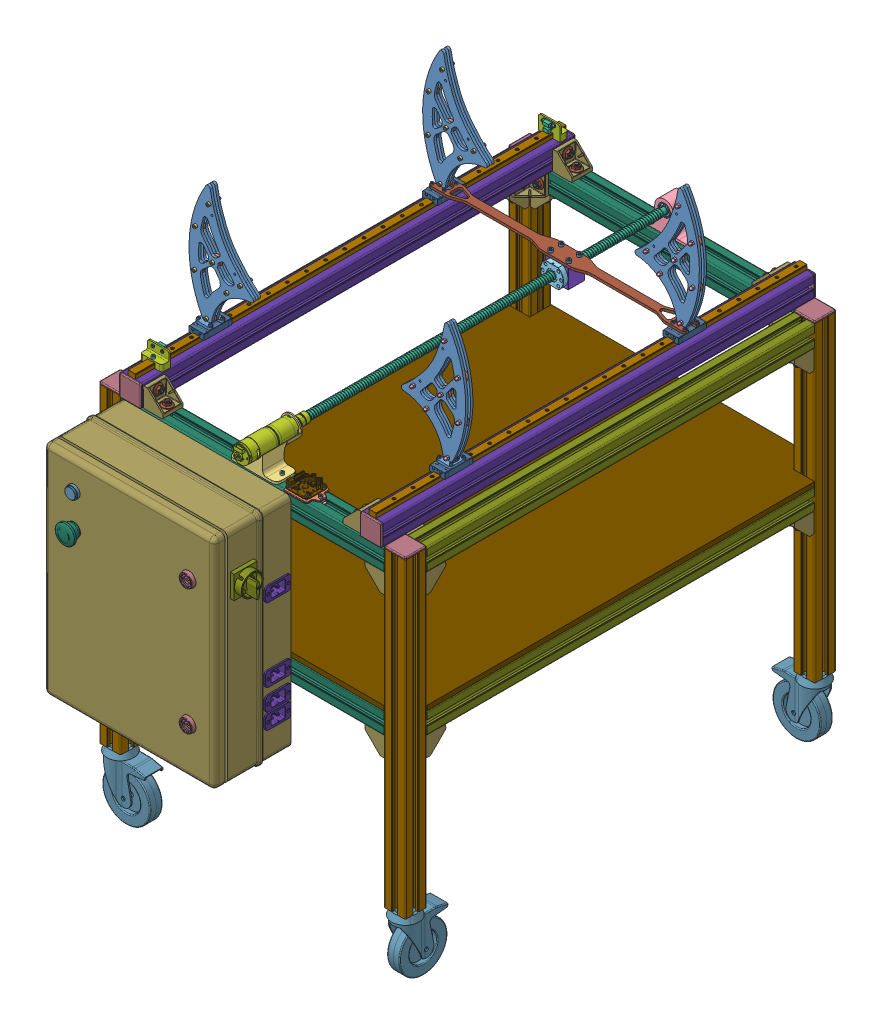
SolidWorks assembly Montaje_Eje_Z, configuration Predeterminado. Lengths in mm.
Overall size (651 1094.15 1088.52).
428 component instances, 43 part files, 191 mates.
Components (placement in the parent):
- socket head cap screw_iso2-2: socket head cap screw_iso2 [ISO 4762 M3 x 8 - 8N] at (-240.4498 15.8322 -56.4995) x (0 -1 0) z (0 0 1) size (11 5.5 5.5)
- socket head cap screw_iso2-3: socket head cap screw_iso2 [ISO 4762 M3 x 8 - 8N] at (-215.4498 15.8322 -31.4995) x (0 -1 0) z (0 0 1) size (11 5.5 5.5)
- socket head cap screw_iso2-4: socket head cap screw_iso2 [ISO 4762 M3 x 8 - 8N] at (-240.4498 15.8322 -31.4995) x (0 -1 0) z (0 0 1) size (11 5.5 5.5)
- socket head cap screw_iso2-5: socket head cap screw_iso2 [ISO 4762 M3 x 8 - 8N] at (-215.4498 15.8322 -56.4995) x (0 -1 0) z (0.194661 0 0.98087) size (11 5.5 5.5)
- socket head cap screw_iso2-6: socket head cap screw_iso2 [ISO 4762 M3 x 8 - 8N] at (287.5502 15.8322 -56.4995) x (0 -1 0) z (0.194661 0 0.98087) size (11 5.5 5.5)
- socket head cap screw_iso2-7: socket head cap screw_iso2 [ISO 4762 M3 x 8 - 8N] at (262.5502 15.8322 -31.4995) x (0 -1 0) z (0 0 1) size (11 5.5 5.5)
- socket head cap screw_iso2-8: socket head cap screw_iso2 [ISO 4762 M3 x 8 - 8N] at (287.5502 15.8322 -31.4995) x (0 -1 0) z (-0.140271 0 0.990113) size (11 5.5 5.5)
- socket head cap screw_iso2-9: socket head cap screw_iso2 [ISO 4762 M3 x 8 - 8N] at (262.5502 15.8322 -56.4995) x (0 -1 0) z (-0.070011 0 0.997546) size (11 5.5 5.5)
- socket head cap screw_iso2-10: socket head cap screw_iso2 [ISO 4762 M5 x 16 - 16N] at (43.5502 17.8322 -54.9995) x (0 -1 0) z (0 0 1) size (21 8.5 8.5)
- socket head cap screw_iso2-11: socket head cap screw_iso2 [ISO 4762 M5 x 16 - 16N] at (43.5502 17.8322 -32.9995) x (0 -1 0) z (0.965322 0 -0.261062) size (21 8.5 8.5)
- socket head cap screw_iso2-12: socket head cap screw_iso2 [ISO 4762 M5 x 16 - 16N] at (5.5502 17.8322 -32.9995) x (0 -1 0) z (0 0 1) size (21 8.5 8.5)
- socket head cap screw_iso2-13: socket head cap screw_iso2 [ISO 4762 M5 x 16 - 16N] at (5.5502 17.8322 -54.9995) x (0 -1 0) z (0 0 1) size (21 8.5 8.5)
- socket head cap screw_iso2-23: socket head cap screw_iso2 [ISO 4762 M3 x 8 - 8N] at (287.5502 15.8322 456.5005) x (0 -1 0) z (0 0 1) size (11 5.5 5.5)
- socket head cap screw_iso2-24: socket head cap screw_iso2 [ISO 4762 M3 x 8 - 8N] at (287.5502 15.8322 431.5005) x (0 -1 0) z (0 0 1) size (11 5.5 5.5)
- socket head cap screw_iso2-25: socket head cap screw_iso2 [ISO 4762 M3 x 8 - 8N] at (262.5502 15.8322 456.5005) x (0 -1 0) z (0 0 1) size (11 5.5 5.5)
- socket head cap screw_iso2-26: socket head cap screw_iso2 [ISO 4762 M3 x 8 - 8N] at (262.5502 15.8322 431.5005) x (0 -1 0) z (0 0 1) size (11 5.5 5.5)
- socket head cap screw_iso2-27: socket head cap screw_iso2 [ISO 4762 M3 x 8 - 8N] at (-240.4501 15.8323 456.5005) x (0 -1 0) z (0 0 1) size (11 5.5 5.5)
- socket head cap screw_iso2-28: socket head cap screw_iso2 [ISO 4762 M3 x 8 - 8N] at (-215.4501 15.8323 456.5005) x (0 -1 0) z (0 0 1) size (11 5.5 5.5)
- socket head cap screw_iso2-29: socket head cap screw_iso2 [ISO 4762 M3 x 8 - 8N] at (-240.4501 15.8323 431.5005) x (0 -1 0) z (0 0 1) size (11 5.5 5.5)
- socket head cap screw_iso2-30: socket head cap screw_iso2 [ISO 4762 M3 x 8 - 8N] at (-215.4501 15.8323 431.5005) x (0 -1 0) z (0 0 1) size (11 5.5 5.5)
- socket head cap screw_iso2-31: socket head cap screw_iso2 [ISO 4762 M4 x 8 - 8N] at (144.6751 -48.9678 586.0585) x (0 -1 0) z (0 0 1) size (12 7 7)
- socket head cap screw_iso2-33: socket head cap screw_iso2 [ISO 4762 M4 x 8 - 8N] at (84.6751 -48.9678 586.0585) x (0 -1 0) z (0 0 1) size (12 7 7)
- hexa csunk flathd screw_iso2-1: hexa csunk flathd screw_iso2 [ISO 14581 M3x12x12-N] at (133.4451 -55.9678 604.7785) x (-0.795034 0 0.606565) z (0 -1 0) size (5.5 5.5 12)
- hexa csunk flathd screw_iso2-2: hexa csunk flathd screw_iso2 [ISO 14581 M3x12x12-N] at (96.0351 -55.9678 604.7785) x (-0.795034 0 0.606565) z (0 -1 0) size (5.5 5.5 12)
- hexa csunk flathd screw_iso2-4: hexa csunk flathd screw_iso2 [ISO 14581 M3x12x12-N] at (133.4451 -55.9678 567.3685) x (-0.795034 0 0.606565) z (0 -1 0) size (5.5 5.5 12)
- hexa csunk flathd screw_iso2-5: hexa csunk flathd screw_iso2 [ISO 14581 M3x12x12-N] at (96.0351 -55.9678 567.3685) x (-0.795034 0 0.606565) z (0 -1 0) size (5.5 5.5 12)
- hex thin nut chamfered gradeab_iso-1: hex thin nut chamfered gradeab_iso [ISO - 4035 - M3 - N] at (96.0351 -46.1293 604.7785) x (0.635839 0 0.771821) z (0 1 0) size (5.5 6.35 1.8)
- hex thin nut chamfered gradeab_iso-2: hex thin nut chamfered gradeab_iso [ISO - 4035 - M3 - N] at (133.4739 -46.1293 604.6517) x (1 0 0) z (0 1 0) size (5.5 6.35 1.8)
- hex thin nut chamfered gradeab_iso-3: hex thin nut chamfered gradeab_iso [ISO - 4035 - M3 - N] at (133.4739 -46.1293 567.2883) x (1 0 0) z (0 1 0) size (5.5 6.35 1.8)
- hex thin nut chamfered gradeab_iso-4: hex thin nut chamfered gradeab_iso [ISO - 4035 - M3 - N] at (96.0597 -46.1293 567.2629) x (1 0 0) z (0 1 0) size (5.5 6.35 1.8)
- bosch_3842530281_56mh0c106byol9t07uu6uwj7k-1: bosch_3842530281_56mh0c106byol9t07uu6uwj7k [Default] at (84.6751 -58.9678 586.0585) x (1 0 0) z (0 0 1) size (19.6 8.7 10)
- bosch_3842530281_56mh0c106byol9t07uu6uwj7k-2: bosch_3842530281_56mh0c106byol9t07uu6uwj7k [Default] at (144.6751 -58.9678 586.0585) x (1 0 0) z (0 0 1) size (19.6 8.7 10)
- bosch_3842530281_56mh0c106byol9t07uu6uwj7k-3: bosch_3842530281_56mh0c106byol9t07uu6uwj7k [Default] at (64.0502 -58.9678 586.0585) x (1 0 0) z (0 0 1) size (19.6 8.7 10)
- bosch_3842530281_56mh0c106byol9t07uu6uwj7k-4: bosch_3842530281_56mh0c106byol9t07uu6uwj7k [Default] at (-14.9498 -58.9678 586.0585) x (1 0 0) z (0 0 1) size (19.6 8.7 10)
- socket head cap screw_iso-1: socket head cap screw_iso [ISO 4762 M4 x 8 - 8N] at (64.0502 -46.9678 586.0585) x (0 -1 0) z (0 0 1) size (12 7 7)
- socket head cap screw_iso-2: socket head cap screw_iso [ISO 4762 M4 x 8 - 8N] at (-14.9498 -46.9678 586.0585) x (0 -1 0) z (0 0 1) size (12 7 7)
- bosch_3842530281_56mh0c106byol9t07uu6uwj7k-5: bosch_3842530281_56mh0c106byol9t07uu6uwj7k [Default] at (64.5502 -58.9678 -268.9416) x (1 0 0) z (0 0 1) size (19.6 8.7 10)
- bosch_3842530281_56mh0c106byol9t07uu6uwj7k-6: bosch_3842530281_56mh0c106byol9t07uu6uwj7k [Default] at (-15.4498 -58.9678 -268.9416) x (1 0 0) z (0 0 1) size (19.6 8.7 10)
- socket head cap screw_iso-3: socket head cap screw_iso [ISO 4762 M4 x 8 - 8N] at (64.5502 -46.9678 -268.9416) x (0 -1 0) z (0 0 1) size (12 7 7)
- socket head cap screw_iso-4: socket head cap screw_iso [ISO 4762 M4 x 8 - 8N] at (-15.4498 -46.9678 -268.9416) x (0 -1 0) z (0 0 1) size (12 7 7)
- bosch_3842530281_56mh0c106byol9t07uu6uwj7k-7: bosch_3842530281_56mh0c106byol9t07uu6uwj7k [Default] at (-227.9501 -13.9677 -276.5915) x (0 0 1) z (-1 0 0) size (19.6 8.7 10)
- bosch_3842530281_56mh0c106byol9t07uu6uwj7k-8: bosch_3842530281_56mh0c106byol9t07uu6uwj7k [Default] at (-227.9501 -13.9677 563.4085) x (0 0 1) z (-1 0 0) size (19.6 8.7 10)
- bosch_3842530281_56mh0c106byol9t07uu6uwj7k-9: bosch_3842530281_56mh0c106byol9t07uu6uwj7k [Default] at (275.0502 -13.9677 563.7084) x (0 0 -1) z (1 0 0) size (19.6 8.7 10)
- bosch_3842530281_56mh0c106byol9t07uu6uwj7k-10: bosch_3842530281_56mh0c106byol9t07uu6uwj7k [Default] at (275.0502 -13.9677 -276.2916) x (0.798528 0 0.601957) z (-0.601957 0 0.798528) size (19.6 8.7 10)
- socket head cap screw_iso-5: socket head cap screw_iso [ISO 4762 M4 x 16 - 16N] at (-227.9501 6.0323 -276.5915) x (0 -1 0) z (0 0 1) size (20 7 7)
- socket head cap screw_iso-8: socket head cap screw_iso [ISO 4762 M3 x 8 - 8N] at (-237.9501 14.0323 -258.9915) x (0 0 -1) z (1 0 0) size (11 5.5 5.5)
- socket head cap screw_iso-9: socket head cap screw_iso [ISO 4762 M3 x 8 - 8N] at (-217.9501 14.0323 -258.9915) x (0 0 -1) z (1 0 0) size (11 5.5 5.5)
- socket head cap screw_iso-10: socket head cap screw_iso [ISO 4762 M3 x 8 - 8N] at (-217.9501 14.0323 545.8085) x (0 0 1) z (0.923728 0.383049 0) size (11 5.5 5.5)
- socket head cap screw_iso-11: socket head cap screw_iso [ISO 4762 M3 x 8 - 8N] at (-237.9501 14.0323 545.8085) x (0 0 1) z (0.923728 0.383049 0) size (11 5.5 5.5)
- socket head cap screw_iso-12: socket head cap screw_iso [ISO 4762 M4 x 16 - 16N] at (-227.9501 6.0323 563.4085) x (0 -1 0) z (0 0 1) size (20 7 7)
- hex thin nut gradeb_iso-1: hex thin nut gradeb_iso [ISO - 4036 - M3 - N] at (-237.9501 14.0323 555.2085) x (1 0 0) z (0 0 1) size (5.5 6.35 1.8)
- hex thin nut gradeb_iso-2: hex thin nut gradeb_iso [ISO - 4036 - M3 - N] at (-217.9501 14.0323 555.2085) x (1 0 0) z (0 0 1) size (5.5 6.35 1.8)
- hex thin nut gradeb_iso-3: hex thin nut gradeb_iso [ISO - 4036 - M3 - N] at (-237.9501 14.0323 -268.3915) x (-1 -0.000019 0) z (0 0 -1) size (5.5 6.35 1.8)
- hex thin nut gradeb_iso-4: hex thin nut gradeb_iso [ISO - 4036 - M3 - N] at (-217.9501 14.0323 -268.3915) x (-1 -0.000027 0) z (0 0 -1) size (5.5 6.35 1.8)
- Motor_Tornillos-1: Motor_Tornillos [Predeterminado] at (24.5502 -12.1678 506.5645) x (-1 0 0) z (0 0 -1) size (37.2 37.03 132.01)
  - Motor_Tornillos.CATProduct-1: Motor_Tornillos.CATProduct [Predeterminado] at origin size (37.2 37.03 132.01)
    - CHP-36GP-555.CATPart-1: CHP-36GP-555.CATPart [Predeterminado] at (0 0 -31.394) size (37.2 37.03 132.01)
    - ISO_4762_M3x12_STEEL_HEXAGON_SOCKET_HEAD_CAP_SCREW.CATPart-1: ISO_4762_M3x12_STEEL_HEXAGON_SOCKET_HEAD_CAP_SCREW.CATPart [Predeterminado] at (-9.8995 -9.8995 -17.394) x (0 0 1) z (1 0 0) size (15 5.5 5.5)
    - Gathered ISO 4762 SCREW M3x12 STEEL HEXAGON SOCKET HEAD CAP on CircPattern.7.CATProduct-1: Gathered ISO 4762 SCREW M3x12 STEEL HEXAGON SOCKET HEAD CAP on CircPattern.7.CATProduct [Predeterminado] at origin size (25.3 25.3 15)
      - ISO_4762_M3x12_STEEL_HEXAGON_SOCKET_HEAD_CAP_SCREW.CATPart-1: ISO_4762_M3x12_STEEL_HEXAGON_SOCKET_HEAD_CAP_SCREW.CATPart [Predeterminado] at (9.8995 9.8995 -17.394) x (0 0 1) z (-1 0 0) size (15 5.5 5.5)
      - ISO_4762_M3x12_STEEL_HEXAGON_SOCKET_HEAD_CAP_SCREW.CATPart-2: ISO_4762_M3x12_STEEL_HEXAGON_SOCKET_HEAD_CAP_SCREW.CATPart [Predeterminado] at (-9.8995 9.8995 -17.394) x (0 0 1) z (0 -1 0) size (15 5.5 5.5)
      - ISO_4762_M3x12_STEEL_HEXAGON_SOCKET_HEAD_CAP_SCREW.CATPart-3: ISO_4762_M3x12_STEEL_HEXAGON_SOCKET_HEAD_CAP_SCREW.CATPart [Predeterminado] at (9.8995 -9.8995 -17.394) x (0 0 1) z (0 1 0) size (15 5.5 5.5)
- Montaje_Mesa.CATProduct-1: Montaje_Mesa.CATProduct [Predeterminado] at (176.75 -638.9678 608.5583) x (1 0 0) z (0 1 0) size (651 911 824)
  - Montaje_Pata.CATProduct-1: Montaje_Pata.CATProduct [Predeterminado] at (124.8 44.6853 -67) size (91.5 103 783)
    - P45L_N10_B_650.CATPart-1: P45L_N10_B_650.CATPart [Predeterminado] at (0 0.3146 0) size (45 45 650)
    - Montaje_Escuadra.CATProduct-1: Montaje_Escuadra.CATProduct [Predeterminado] at (19.5001 29.5936 661.8715) x (0 -1 0) z (0 0 -1) size (52 42 52)
      - Tornillo_M8_Martillo.CATPart-1: Tornillo_M8_Martillo.CATPart [Predeterminado] at (0.029 0 50.8715) size (8.5 19 30)
      - Tuerca_M8.CATPart-1: Tuerca_M8.CATPart [Predeterminado] at (0.029 0 66.3715) size (21 21 8)
      - Bracket_45_B-Type_slot_10.CATPart-1: Bracket_45_B-Type_slot_10.CATPart [Predeterminado] at (29.279 0 56.8715) x (0 1 0) z (0 0 1) size (42 44.89 44.89)
      - Tuerca_M8.CATPart-2: Tuerca_M8.CATPart [Predeterminado] at (19.779 0 86.1215) x (0 0 1) z (-1 0 0) size (21 21 8)
      - Tornillo_M8_Martillo.CATPart-2: Tornillo_M8_Martillo.CATPart [Predeterminado] at (35.279 0 86.1215) x (0 0 1) z (-1 0 0) size (8.5 19 30)
    - Montaje_Escuadra.CATProduct-2: Montaje_Escuadra.CATProduct [Predeterminado] at (53.8716 -22.1855 575.721) x (0 0 1) z (-1 0 0) size (52 42 52)
      - Tornillo_M8_Martillo.CATPart-1: Tornillo_M8_Martillo.CATPart [Predeterminado] at (0.029 0 50.8715) size (8.5 19 30)
      - Tuerca_M8.CATPart-1: Tuerca_M8.CATPart [Predeterminado] at (0.029 0 66.3715) size (21 21 8)
      - Bracket_45_B-Type_slot_10.CATPart-1: Bracket_45_B-Type_slot_10.CATPart [Predeterminado] at (29.279 0 56.8715) x (0 1 0) z (0 0 1) size (42 44.89 44.89)
      - Tuerca_M8.CATPart-2: Tuerca_M8.CATPart [Predeterminado] at (19.779 0 86.1215) x (0 0 1) z (-1 0 0) size (21 21 8)
      - Tornillo_M8_Martillo.CATPart-2: Tornillo_M8_Martillo.CATPart [Predeterminado] at (35.279 0 86.1215) x (0 0 1) z (-1 0 0) size (8.5 19 30)
    - Montaje_Escuadra.CATProduct-3: Montaje_Escuadra.CATProduct [Predeterminado] at (19.5001 29.5936 366.8715) x (0 -1 0) z (0 0 -1) size (52 42 52)
      - Tornillo_M8_Martillo.CATPart-1: Tornillo_M8_Martillo.CATPart [Predeterminado] at (0.029 0 50.8715) size (8.5 19 30)
      - Tuerca_M8.CATPart-1: Tuerca_M8.CATPart [Predeterminado] at (0.029 0 66.3715) size (21 21 8)
      - Bracket_45_B-Type_slot_10.CATPart-1: Bracket_45_B-Type_slot_10.CATPart [Predeterminado] at (29.279 0 56.8715) x (0 1 0) z (0 0 1) size (42 44.89 44.89)
      - Tuerca_M8.CATPart-2: Tuerca_M8.CATPart [Predeterminado] at (19.779 0 86.1215) x (0 0 1) z (-1 0 0) size (21 21 8)
      - Tornillo_M8_Martillo.CATPart-2: Tornillo_M8_Martillo.CATPart [Predeterminado] at (35.279 0 86.1215) x (0 0 1) z (-1 0 0) size (8.5 19 30)
    - Montaje_Escuadra.CATProduct-4: Montaje_Escuadra.CATProduct [Predeterminado] at (53.8716 -22.1855 280.721) x (0 0 1) z (-1 0 0) size (52 42 52)
      - Tornillo_M8_Martillo.CATPart-1: Tornillo_M8_Martillo.CATPart [Predeterminado] at (0.029 0 50.8715) size (8.5 19 30)
      - Tuerca_M8.CATPart-1: Tuerca_M8.CATPart [Predeterminado] at (0.029 0 66.3715) size (21 21 8)
      - Bracket_45_B-Type_slot_10.CATPart-1: Bracket_45_B-Type_slot_10.CATPart [Predeterminado] at (29.279 0 56.8715) x (0 1 0) z (0 0 1) size (42 44.89 44.89)
      - Tuerca_M8.CATPart-2: Tuerca_M8.CATPart [Predeterminado] at (19.779 0 86.1215) x (0 0 1) z (-1 0 0) size (21 21 8)
      - Tornillo_M8_Martillo.CATPart-2: Tornillo_M8_Martillo.CATPart [Predeterminado] at (35.279 0 86.1215) x (0 0 1) z (-1 0 0) size (8.5 19 30)
    - Tapa 45x45.CATPart-1: Tapa 45x45.CATPart [Predeterminado] at (19.5002 -22.1854 650) size (45 45 4)
    - Rueda100mm.CATPart-1: Rueda100mm.CATPart [Predeterminado] at (19.5001 2.8145 -79) x (0 -1 0) z (0 0 1) size (103 56 129)
  - P45L_N10_B_550.CATPart-1: P45L_N10_B_550.CATPart [Predeterminado] at (-428.2 44.9998 580) x (0 0 -1) z (1 0 0) size (45 45 550)
  - P45L_N10_B_810.CATPart-1: P45L_N10_B_810.CATPart [Predeterminado] at (124.8 854.9998 583) x (1 0 0) z (0 -1 0) size (45 45 810)
  - Montaje_Pata.CATProduct-2: Montaje_Pata.CATProduct [Predeterminado] at (-428.5146 41.9998 -67) x (0 -1 0) z (0 0 1) size (91.5 103 783)
    - P45L_N10_B_650.CATPart-1: P45L_N10_B_650.CATPart [Predeterminado] at (0 0.3146 0) size (45 45 650)
    - Montaje_Escuadra.CATProduct-1: Montaje_Escuadra.CATProduct [Predeterminado] at (19.5001 29.5936 661.8715) x (0 -1 0) z (0 0 -1) size (52 42 52)
      - Tornillo_M8_Martillo.CATPart-1: Tornillo_M8_Martillo.CATPart [Predeterminado] at (0.029 0 50.8715) size (8.5 19 30)
      - Tuerca_M8.CATPart-1: Tuerca_M8.CATPart [Predeterminado] at (0.029 0 66.3715) size (21 21 8)
      - Bracket_45_B-Type_slot_10.CATPart-1: Bracket_45_B-Type_slot_10.CATPart [Predeterminado] at (29.279 0 56.8715) x (0 1 0) z (0 0 1) size (42 44.89 44.89)
      - Tuerca_M8.CATPart-2: Tuerca_M8.CATPart [Predeterminado] at (19.779 0 86.1215) x (0 0 1) z (-1 0 0) size (21 21 8)
      - Tornillo_M8_Martillo.CATPart-2: Tornillo_M8_Martillo.CATPart [Predeterminado] at (35.279 0 86.1215) x (0 0 1) z (-1 0 0) size (8.5 19 30)
    - Montaje_Escuadra.CATProduct-2: Montaje_Escuadra.CATProduct [Predeterminado] at (53.8716 -22.1855 575.721) x (0 0 1) z (-1 0 0) size (52 42 52)
      - Tornillo_M8_Martillo.CATPart-1: Tornillo_M8_Martillo.CATPart [Predeterminado] at (0.029 0 50.8715) size (8.5 19 30)
      - Tuerca_M8.CATPart-1: Tuerca_M8.CATPart [Predeterminado] at (0.029 0 66.3715) size (21 21 8)
      - Bracket_45_B-Type_slot_10.CATPart-1: Bracket_45_B-Type_slot_10.CATPart [Predeterminado] at (29.279 0 56.8715) x (0 1 0) z (0 0 1) size (42 44.89 44.89)
      - Tuerca_M8.CATPart-2: Tuerca_M8.CATPart [Predeterminado] at (19.779 0 86.1215) x (0 0 1) z (-1 0 0) size (21 21 8)
      - Tornillo_M8_Martillo.CATPart-2: Tornillo_M8_Martillo.CATPart [Predeterminado] at (35.279 0 86.1215) x (0 0 1) z (-1 0 0) size (8.5 19 30)
    - Montaje_Escuadra.CATProduct-3: Montaje_Escuadra.CATProduct [Predeterminado] at (19.5001 29.5936 366.8715) x (0 -1 0) z (0 0 -1) size (52 42 52)
      - Tornillo_M8_Martillo.CATPart-1: Tornillo_M8_Martillo.CATPart [Predeterminado] at (0.029 0 50.8715) size (8.5 19 30)
      - Tuerca_M8.CATPart-1: Tuerca_M8.CATPart [Predeterminado] at (0.029 0 66.3715) size (21 21 8)
      - Bracket_45_B-Type_slot_10.CATPart-1: Bracket_45_B-Type_slot_10.CATPart [Predeterminado] at (29.279 0 56.8715) x (0 1 0) z (0 0 1) size (42 44.89 44.89)
      - Tuerca_M8.CATPart-2: Tuerca_M8.CATPart [Predeterminado] at (19.779 0 86.1215) x (0 0 1) z (-1 0 0) size (21 21 8)
      - Tornillo_M8_Martillo.CATPart-2: Tornillo_M8_Martillo.CATPart [Predeterminado] at (35.279 0 86.1215) x (0 0 1) z (-1 0 0) size (8.5 19 30)
    - Montaje_Escuadra.CATProduct-4: Montaje_Escuadra.CATProduct [Predeterminado] at (53.8716 -22.1855 280.721) x (0 0 1) z (-1 0 0) size (52 42 52)
      - Tornillo_M8_Martillo.CATPart-1: Tornillo_M8_Martillo.CATPart [Predeterminado] at (0.029 0 50.8715) size (8.5 19 30)
      - Tuerca_M8.CATPart-1: Tuerca_M8.CATPart [Predeterminado] at (0.029 0 66.3715) size (21 21 8)
      - Bracket_45_B-Type_slot_10.CATPart-1: Bracket_45_B-Type_slot_10.CATPart [Predeterminado] at (29.279 0 56.8715) x (0 1 0) z (0 0 1) size (42 44.89 44.89)
      - Tuerca_M8.CATPart-2: Tuerca_M8.CATPart [Predeterminado] at (19.779 0 86.1215) x (0 0 1) z (-1 0 0) size (21 21 8)
      - Tornillo_M8_Martillo.CATPart-2: Tornillo_M8_Martillo.CATPart [Predeterminado] at (35.279 0 86.1215) x (0 0 1) z (-1 0 0) size (8.5 19 30)
    - Tapa 45x45.CATPart-1: Tapa 45x45.CATPart [Predeterminado] at (19.5002 -22.1854 650) size (45 45 4)
    - Rueda100mm.CATPart-1: Rueda100mm.CATPart [Predeterminado] at (19.5001 2.8145 -79) x (0 -1 0) z (0 0 1) size (103 56 129)
  - Montaje_Pata.CATProduct-3: Montaje_Pata.CATProduct [Predeterminado] at (122.1146 857.9998 -67) x (0 1 0) z (0 0 1) size (91.5 103 783)
    - P45L_N10_B_650.CATPart-1: P45L_N10_B_650.CATPart [Predeterminado] at (0 0.3146 0) size (45 45 650)
    - Montaje_Escuadra.CATProduct-1: Montaje_Escuadra.CATProduct [Predeterminado] at (19.5001 29.5936 661.8715) x (0 -1 0) z (0 0 -1) size (52 42 52)
      - Tornillo_M8_Martillo.CATPart-1: Tornillo_M8_Martillo.CATPart [Predeterminado] at (0.029 0 50.8715) size (8.5 19 30)
      - Tuerca_M8.CATPart-1: Tuerca_M8.CATPart [Predeterminado] at (0.029 0 66.3715) size (21 21 8)
      - Bracket_45_B-Type_slot_10.CATPart-1: Bracket_45_B-Type_slot_10.CATPart [Predeterminado] at (29.279 0 56.8715) x (0 1 0) z (0 0 1) size (42 44.89 44.89)
      - Tuerca_M8.CATPart-2: Tuerca_M8.CATPart [Predeterminado] at (19.779 0 86.1215) x (0 0 1) z (-1 0 0) size (21 21 8)
      - Tornillo_M8_Martillo.CATPart-2: Tornillo_M8_Martillo.CATPart [Predeterminado] at (35.279 0 86.1215) x (0 0 1) z (-1 0 0) size (8.5 19 30)
    - Montaje_Escuadra.CATProduct-2: Montaje_Escuadra.CATProduct [Predeterminado] at (53.8716 -22.1855 575.721) x (0 0 1) z (-1 0 0) size (52 42 52)
      - Tornillo_M8_Martillo.CATPart-1: Tornillo_M8_Martillo.CATPart [Predeterminado] at (0.029 0 50.8715) size (8.5 19 30)
      - Tuerca_M8.CATPart-1: Tuerca_M8.CATPart [Predeterminado] at (0.029 0 66.3715) size (21 21 8)
      - Bracket_45_B-Type_slot_10.CATPart-1: Bracket_45_B-Type_slot_10.CATPart [Predeterminado] at (29.279 0 56.8715) x (0 1 0) z (0 0 1) size (42 44.89 44.89)
      - Tuerca_M8.CATPart-2: Tuerca_M8.CATPart [Predeterminado] at (19.779 0 86.1215) x (0 0 1) z (-1 0 0) size (21 21 8)
      - Tornillo_M8_Martillo.CATPart-2: Tornillo_M8_Martillo.CATPart [Predeterminado] at (35.279 0 86.1215) x (0 0 1) z (-1 0 0) size (8.5 19 30)
    - Montaje_Escuadra.CATProduct-3: Montaje_Escuadra.CATProduct [Predeterminado] at (19.5001 29.5936 366.8715) x (0 -1 0) z (0 0 -1) size (52 42 52)
      - Tornillo_M8_Martillo.CATPart-1: Tornillo_M8_Martillo.CATPart [Predeterminado] at (0.029 0 50.8715) size (8.5 19 30)
      - Tuerca_M8.CATPart-1: Tuerca_M8.CATPart [Predeterminado] at (0.029 0 66.3715) size (21 21 8)
      - Bracket_45_B-Type_slot_10.CATPart-1: Bracket_45_B-Type_slot_10.CATPart [Predeterminado] at (29.279 0 56.8715) x (0 1 0) z (0 0 1) size (42 44.89 44.89)
      - Tuerca_M8.CATPart-2: Tuerca_M8.CATPart [Predeterminado] at (19.779 0 86.1215) x (0 0 1) z (-1 0 0) size (21 21 8)
      - Tornillo_M8_Martillo.CATPart-2: Tornillo_M8_Martillo.CATPart [Predeterminado] at (35.279 0 86.1215) x (0 0 1) z (-1 0 0) size (8.5 19 30)
    - Montaje_Escuadra.CATProduct-4: Montaje_Escuadra.CATProduct [Predeterminado] at (53.8716 -22.1855 280.721) x (0 0 1) z (-1 0 0) size (52 42 52)
      - Tornillo_M8_Martillo.CATPart-1: Tornillo_M8_Martillo.CATPart [Predeterminado] at (0.029 0 50.8715) size (8.5 19 30)
      - Tuerca_M8.CATPart-1: Tuerca_M8.CATPart [Predeterminado] at (0.029 0 66.3715) size (21 21 8)
      - Bracket_45_B-Type_slot_10.CATPart-1: Bracket_45_B-Type_slot_10.CATPart [Predeterminado] at (29.279 0 56.8715) x (0 1 0) z (0 0 1) size (42 44.89 44.89)
      - Tuerca_M8.CATPart-2: Tuerca_M8.CATPart [Predeterminado] at (19.779 0 86.1215) x (0 0 1) z (-1 0 0) size (21 21 8)
      - Tornillo_M8_Martillo.CATPart-2: Tornillo_M8_Martillo.CATPart [Predeterminado] at (35.279 0 86.1215) x (0 0 1) z (-1 0 0) size (8.5 19 30)
    - Tapa 45x45.CATPart-1: Tapa 45x45.CATPart [Predeterminado] at (19.5002 -22.1854 650) size (45 45 4)
    - Rueda100mm.CATPart-1: Rueda100mm.CATPart [Predeterminado] at (19.5001 2.8145 -79) x (0 -1 0) z (0 0 1) size (103 56 129)
  - P45L_N10_B_810.CATPart-2: P45L_N10_B_810.CATPart [Predeterminado] at (-470.2002 854.9998 583) x (1 0 0) z (0 -1 0) size (45 45 810)
  - P45L_N10_B_550.CATPart-2: P45L_N10_B_550.CATPart [Predeterminado] at (-428.2 900 580) x (0 0 -1) z (1 0 0) size (45 45 550)
  - Montaje_Pata.CATProduct-4: Montaje_Pata.CATProduct [Predeterminado] at (-431.2 855.3144 -67) x (-1 0 0) z (0 0 1) size (91.5 103 783)
    - P45L_N10_B_650.CATPart-1: P45L_N10_B_650.CATPart [Predeterminado] at (0 0.3146 0) size (45 45 650)
    - Montaje_Escuadra.CATProduct-1: Montaje_Escuadra.CATProduct [Predeterminado] at (19.5001 29.5936 661.8715) x (0 -1 0) z (0 0 -1) size (52 42 52)
      - Tornillo_M8_Martillo.CATPart-1: Tornillo_M8_Martillo.CATPart [Predeterminado] at (0.029 0 50.8715) size (8.5 19 30)
      - Tuerca_M8.CATPart-1: Tuerca_M8.CATPart [Predeterminado] at (0.029 0 66.3715) size (21 21 8)
      - Bracket_45_B-Type_slot_10.CATPart-1: Bracket_45_B-Type_slot_10.CATPart [Predeterminado] at (29.279 0 56.8715) x (0 1 0) z (0 0 1) size (42 44.89 44.89)
      - Tuerca_M8.CATPart-2: Tuerca_M8.CATPart [Predeterminado] at (19.779 0 86.1215) x (0 0 1) z (-1 0 0) size (21 21 8)
      - Tornillo_M8_Martillo.CATPart-2: Tornillo_M8_Martillo.CATPart [Predeterminado] at (35.279 0 86.1215) x (0 0 1) z (-1 0 0) size (8.5 19 30)
    - Montaje_Escuadra.CATProduct-2: Montaje_Escuadra.CATProduct [Predeterminado] at (53.8716 -22.1855 575.721) x (0 0 1) z (-1 0 0) size (52 42 52)
      - Tornillo_M8_Martillo.CATPart-1: Tornillo_M8_Martillo.CATPart [Predeterminado] at (0.029 0 50.8715) size (8.5 19 30)
      - Tuerca_M8.CATPart-1: Tuerca_M8.CATPart [Predeterminado] at (0.029 0 66.3715) size (21 21 8)
      - Bracket_45_B-Type_slot_10.CATPart-1: Bracket_45_B-Type_slot_10.CATPart [Predeterminado] at (29.279 0 56.8715) x (0 1 0) z (0 0 1) size (42 44.89 44.89)
      - Tuerca_M8.CATPart-2: Tuerca_M8.CATPart [Predeterminado] at (19.779 0 86.1215) x (0 0 1) z (-1 0 0) size (21 21 8)
      - Tornillo_M8_Martillo.CATPart-2: Tornillo_M8_Martillo.CATPart [Predeterminado] at (35.279 0 86.1215) x (0 0 1) z (-1 0 0) size (8.5 19 30)
    - Montaje_Escuadra.CATProduct-3: Montaje_Escuadra.CATProduct [Predeterminado] at (19.5001 29.5936 366.8715) x (0 -1 0) z (0 0 -1) size (52 42 52)
      - Tornillo_M8_Martillo.CATPart-1: Tornillo_M8_Martillo.CATPart [Predeterminado] at (0.029 0 50.8715) size (8.5 19 30)
      - Tuerca_M8.CATPart-1: Tuerca_M8.CATPart [Predeterminado] at (0.029 0 66.3715) size (21 21 8)
      - Bracket_45_B-Type_slot_10.CATPart-1: Bracket_45_B-Type_slot_10.CATPart [Predeterminado] at (29.279 0 56.8715) x (0 1 0) z (0 0 1) size (42 44.89 44.89)
      - Tuerca_M8.CATPart-2: Tuerca_M8.CATPart [Predeterminado] at (19.779 0 86.1215) x (0 0 1) z (-1 0 0) size (21 21 8)
      - Tornillo_M8_Martillo.CATPart-2: Tornillo_M8_Martillo.CATPart [Predeterminado] at (35.279 0 86.1215) x (0 0 1) z (-1 0 0) size (8.5 19 30)
    - Montaje_Escuadra.CATProduct-4: Montaje_Escuadra.CATProduct [Predeterminado] at (53.8716 -22.1855 280.721) x (0 0 1) z (-1 0 0) size (52 42 52)
      - Tornillo_M8_Martillo.CATPart-1: Tornillo_M8_Martillo.CATPart [Predeterminado] at (0.029 0 50.8715) size (8.5 19 30)
      - Tuerca_M8.CATPart-1: Tuerca_M8.CATPart [Predeterminado] at (0.029 0 66.3715) size (21 21 8)
      - Bracket_45_B-Type_slot_10.CATPart-1: Bracket_45_B-Type_slot_10.CATPart [Predeterminado] at (29.279 0 56.8715) x (0 1 0) z (0 0 1) size (42 44.89 44.89)
      - Tuerca_M8.CATPart-2: Tuerca_M8.CATPart [Predeterminado] at (19.779 0 86.1215) x (0 0 1) z (-1 0 0) size (21 21 8)
      - Tornillo_M8_Martillo.CATPart-2: Tornillo_M8_Martillo.CATPart [Predeterminado] at (35.279 0 86.1215) x (0 0 1) z (-1 0 0) size (8.5 19 30)
    - Tapa 45x45.CATPart-1: Tapa 45x45.CATPart [Predeterminado] at (19.5002 -22.1854 650) size (45 45 4)
    - Rueda100mm.CATPart-1: Rueda100mm.CATPart [Predeterminado] at (19.5001 2.8145 -79) x (0 -1 0) z (0 0 1) size (103 56 129)
  - P45L_N10_B_550.CATPart-3: P45L_N10_B_550.CATPart [Predeterminado] at (-428.2 900 284.9998) x (0 0 -1) z (1 0 0) size (45 45 550)
  - P45L_N10_B_810.CATPart-3: P45L_N10_B_810.CATPart [Predeterminado] at (-470.2002 854.9998 287.9998) x (1 0 0) z (0 -1 0) size (45 45 810)
  - P45L_N10_B_810.CATPart-4: P45L_N10_B_810.CATPart [Predeterminado] at (124.8 854.9998 287.9998) x (1 0 0) z (0 -1 0) size (45 45 810)
  - P45L_N10_B_550.CATPart-4: P45L_N10_B_550.CATPart [Predeterminado] at (-428.2 44.9998 284.9998) x (0 0 -1) z (1 0 0) size (45 45 550)
  - Montaje_Carril.CATProduct-1: Montaje_Carril.CATProduct [Predeterminado] at (75.8 899.85 586) x (0 0 1) z (0 -1 0) size (56 86 908)
    - P45L_N10_B_900.CATPart-1: P45L_N10_B_900.CATPart [Predeterminado] at origin size (45 45 900)
    - Montaje_Escuadra.CATProduct-1: Montaje_Escuadra.CATProduct [Predeterminado] at (-59.8715 29.279 22.35) x (0 -1 0) z (1 0 0) size (52 42 52)
      - Tornillo_M8_Martillo.CATPart-1: Tornillo_M8_Martillo.CATPart [Predeterminado] at (0.029 0 50.8715) size (8.5 19 30)
      - Tuerca_M8.CATPart-1: Tuerca_M8.CATPart [Predeterminado] at (0.029 0 66.3715) size (21 21 8)
      - Bracket_45_B-Type_slot_10.CATPart-1: Bracket_45_B-Type_slot_10.CATPart [Predeterminado] at (29.279 0 56.8715) x (0 1 0) z (0 0 1) size (42 44.89 44.89)
      - Tuerca_M8.CATPart-2: Tuerca_M8.CATPart [Predeterminado] at (19.779 0 86.1215) x (0 0 1) z (-1 0 0) size (21 21 8)
      - Tornillo_M8_Martillo.CATPart-2: Tornillo_M8_Martillo.CATPart [Predeterminado] at (35.279 0 86.1215) x (0 0 1) z (-1 0 0) size (8.5 19 30)
    - Montaje_Escuadra.CATProduct-2: Montaje_Escuadra.CATProduct [Predeterminado] at (-59.8715 29.279 877.5) x (0 -1 0) z (1 0 0) size (52 42 52)
      - Tornillo_M8_Martillo.CATPart-1: Tornillo_M8_Martillo.CATPart [Predeterminado] at (0.029 0 50.8715) size (8.5 19 30)
      - Tuerca_M8.CATPart-1: Tuerca_M8.CATPart [Predeterminado] at (0.029 0 66.3715) size (21 21 8)
      - Bracket_45_B-Type_slot_10.CATPart-1: Bracket_45_B-Type_slot_10.CATPart [Predeterminado] at (29.279 0 56.8715) x (0 1 0) z (0 0 1) size (42 44.89 44.89)
      - Tuerca_M8.CATPart-2: Tuerca_M8.CATPart [Predeterminado] at (19.779 0 86.1215) x (0 0 1) z (-1 0 0) size (21 21 8)
      - Tornillo_M8_Martillo.CATPart-2: Tornillo_M8_Martillo.CATPart [Predeterminado] at (35.279 0 86.1215) x (0 0 1) z (-1 0 0) size (8.5 19 30)
    - Tapa 45x45.CATPart-1: Tapa 45x45.CATPart [Predeterminado] at (19.5 -22.5 0) x (1 0 0) z (0 0 -1) size (45 45 4)
    - Tapa 45x45.CATPart-2: Tapa 45x45.CATPart [Predeterminado] at (19.5 -22.5 900) size (45 45 4)
  - Montaje_Carril.CATProduct-2: Montaje_Carril.CATProduct [Predeterminado] at (-382.2 0.1498 586) x (0 0 1) z (0 1 0) size (56 86 908)
    - P45L_N10_B_900.CATPart-1: P45L_N10_B_900.CATPart [Predeterminado] at origin size (45 45 900)
    - Montaje_Escuadra.CATProduct-1: Montaje_Escuadra.CATProduct [Predeterminado] at (-59.8715 29.279 22.35) x (0 -1 0) z (1 0 0) size (52 42 52)
      - Tornillo_M8_Martillo.CATPart-1: Tornillo_M8_Martillo.CATPart [Predeterminado] at (0.029 0 50.8715) size (8.5 19 30)
      - Tuerca_M8.CATPart-1: Tuerca_M8.CATPart [Predeterminado] at (0.029 0 66.3715) size (21 21 8)
      - Bracket_45_B-Type_slot_10.CATPart-1: Bracket_45_B-Type_slot_10.CATPart [Predeterminado] at (29.279 0 56.8715) x (0 1 0) z (0 0 1) size (42 44.89 44.89)
      - Tuerca_M8.CATPart-2: Tuerca_M8.CATPart [Predeterminado] at (19.779 0 86.1215) x (0 0 1) z (-1 0 0) size (21 21 8)
      - Tornillo_M8_Martillo.CATPart-2: Tornillo_M8_Martillo.CATPart [Predeterminado] at (35.279 0 86.1215) x (0 0 1) z (-1 0 0) size (8.5 19 30)
    - Montaje_Escuadra.CATProduct-2: Montaje_Escuadra.CATProduct [Predeterminado] at (-59.8715 29.279 877.5) x (0 -1 0) z (1 0 0) size (52 42 52)
      - Tornillo_M8_Martillo.CATPart-1: Tornillo_M8_Martillo.CATPart [Predeterminado] at (0.029 0 50.8715) size (8.5 19 30)
      - Tuerca_M8.CATPart-1: Tuerca_M8.CATPart [Predeterminado] at (0.029 0 66.3715) size (21 21 8)
      - Bracket_45_B-Type_slot_10.CATPart-1: Bracket_45_B-Type_slot_10.CATPart [Predeterminado] at (29.279 0 56.8715) x (0 1 0) z (0 0 1) size (42 44.89 44.89)
      - Tuerca_M8.CATPart-2: Tuerca_M8.CATPart [Predeterminado] at (19.779 0 86.1215) x (0 0 1) z (-1 0 0) size (21 21 8)
      - Tornillo_M8_Martillo.CATPart-2: Tornillo_M8_Martillo.CATPart [Predeterminado] at (35.279 0 86.1215) x (0 0 1) z (-1 0 0) size (8.5 19 30)
    - Tapa 45x45.CATPart-1: Tapa 45x45.CATPart [Predeterminado] at (19.5 -22.5 0) x (1 0 0) z (0 0 -1) size (45 45 4)
    - Tapa 45x45.CATPart-2: Tapa 45x45.CATPart [Predeterminado] at (19.5 -22.5 900) size (45 45 4)
  - Montaje_Escuadra.CATProduct-1: Montaje_Escuadra.CATProduct [Predeterminado] at (178.6715 825.7208 560.5) x (0 1 0) z (-1 0 0) size (52 42 52)
    - Tornillo_M8_Martillo.CATPart-1: Tornillo_M8_Martillo.CATPart [Predeterminado] at (0.029 0 50.8715) size (8.5 19 30)
    - Tuerca_M8.CATPart-1: Tuerca_M8.CATPart [Predeterminado] at (0.029 0 66.3715) size (21 21 8)
    - Bracket_45_B-Type_slot_10.CATPart-1: Bracket_45_B-Type_slot_10.CATPart [Predeterminado] at (29.279 0 56.8715) x (0 1 0) z (0 0 1) size (42 44.89 44.89)
    - Tuerca_M8.CATPart-2: Tuerca_M8.CATPart [Predeterminado] at (19.779 0 86.1215) x (0 0 1) z (-1 0 0) size (21 21 8)
    - Tornillo_M8_Martillo.CATPart-2: Tornillo_M8_Martillo.CATPart [Predeterminado] at (35.279 0 86.1215) x (0 0 1) z (-1 0 0) size (8.5 19 30)
  - Montaje_Escuadra.CATProduct-2: Montaje_Escuadra.CATProduct [Predeterminado] at (-398.921 911.8713 560.5) x (-1 0 0) z (0 -1 0) size (52 42 52)
    - Tornillo_M8_Martillo.CATPart-1: Tornillo_M8_Martillo.CATPart [Predeterminado] at (0.029 0 50.8715) size (8.5 19 30)
    - Tuerca_M8.CATPart-1: Tuerca_M8.CATPart [Predeterminado] at (0.029 0 66.3715) size (21 21 8)
    - Bracket_45_B-Type_slot_10.CATPart-1: Bracket_45_B-Type_slot_10.CATPart [Predeterminado] at (29.279 0 56.8715) x (0 1 0) z (0 0 1) size (42 44.89 44.89)
    - Tuerca_M8.CATPart-2: Tuerca_M8.CATPart [Predeterminado] at (19.779 0 86.1215) x (0 0 1) z (-1 0 0) size (21 21 8)
    - Tornillo_M8_Martillo.CATPart-2: Tornillo_M8_Martillo.CATPart [Predeterminado] at (35.279 0 86.1215) x (0 0 1) z (-1 0 0) size (8.5 19 30)
  - Montaje_Escuadra.CATProduct-3: Montaje_Escuadra.CATProduct [Predeterminado] at (92.521 -11.8716 560.4999) x (1 0 0) z (0 1 0) size (52 42 52)
    - Tornillo_M8_Martillo.CATPart-1: Tornillo_M8_Martillo.CATPart [Predeterminado] at (0.029 0 50.8715) size (8.5 19 30)
    - Tuerca_M8.CATPart-1: Tuerca_M8.CATPart [Predeterminado] at (0.029 0 66.3715) size (21 21 8)
    - Bracket_45_B-Type_slot_10.CATPart-1: Bracket_45_B-Type_slot_10.CATPart [Predeterminado] at (29.279 0 56.8715) x (0 1 0) z (0 0 1) size (42 44.89 44.89)
    - Tuerca_M8.CATPart-2: Tuerca_M8.CATPart [Predeterminado] at (19.779 0 86.1215) x (0 0 1) z (-1 0 0) size (21 21 8)
    - Tornillo_M8_Martillo.CATPart-2: Tornillo_M8_Martillo.CATPart [Predeterminado] at (35.279 0 86.1215) x (0 0 1) z (-1 0 0) size (8.5 19 30)
  - Montaje_Escuadra.CATProduct-4: Montaje_Escuadra.CATProduct [Predeterminado] at (-485.0715 74.2788 560.4999) x (0 -1 0) z (1 0 0) size (52 42 52)
    - Tornillo_M8_Martillo.CATPart-1: Tornillo_M8_Martillo.CATPart [Predeterminado] at (0.029 0 50.8715) size (8.5 19 30)
    - Tuerca_M8.CATPart-1: Tuerca_M8.CATPart [Predeterminado] at (0.029 0 66.3715) size (21 21 8)
    - Bracket_45_B-Type_slot_10.CATPart-1: Bracket_45_B-Type_slot_10.CATPart [Predeterminado] at (29.279 0 56.8715) x (0 1 0) z (0 0 1) size (42 44.89 44.89)
    - Tuerca_M8.CATPart-2: Tuerca_M8.CATPart [Predeterminado] at (19.779 0 86.1215) x (0 0 1) z (-1 0 0) size (21 21 8)
    - Tornillo_M8_Martillo.CATPart-2: Tornillo_M8_Martillo.CATPart [Predeterminado] at (35.279 0 86.1215) x (0 0 1) z (-1 0 0) size (8.5 19 30)
  - Montaje_Escuadra.CATProduct-5: Montaje_Escuadra.CATProduct [Predeterminado] at (178.6715 825.7208 265.4997) x (0 1 0) z (-1 0 0) size (52 42 52)
    - Tornillo_M8_Martillo.CATPart-1: Tornillo_M8_Martillo.CATPart [Predeterminado] at (0.029 0 50.8715) size (8.5 19 30)
    - Tuerca_M8.CATPart-1: Tuerca_M8.CATPart [Predeterminado] at (0.029 0 66.3715) size (21 21 8)
    - Bracket_45_B-Type_slot_10.CATPart-1: Bracket_45_B-Type_slot_10.CATPart [Predeterminado] at (29.279 0 56.8715) x (0 1 0) z (0 0 1) size (42 44.89 44.89)
    - Tuerca_M8.CATPart-2: Tuerca_M8.CATPart [Predeterminado] at (19.779 0 86.1215) x (0 0 1) z (-1 0 0) size (21 21 8)
    - Tornillo_M8_Martillo.CATPart-2: Tornillo_M8_Martillo.CATPart [Predeterminado] at (35.279 0 86.1215) x (0 0 1) z (-1 0 0) size (8.5 19 30)
  - Montaje_Escuadra.CATProduct-6: Montaje_Escuadra.CATProduct [Predeterminado] at (-398.921 911.8713 265.4997) x (-1 0 0) z (0 -1 0) size (52 42 52)
    - Tornillo_M8_Martillo.CATPart-1: Tornillo_M8_Martillo.CATPart [Predeterminado] at (0.029 0 50.8715) size (8.5 19 30)
    - Tuerca_M8.CATPart-1: Tuerca_M8.CATPart [Predeterminado] at (0.029 0 66.3715) size (21 21 8)
    - Bracket_45_B-Type_slot_10.CATPart-1: Bracket_45_B-Type_slot_10.CATPart [Predeterminado] at (29.279 0 56.8715) x (0 1 0) z (0 0 1) size (42 44.89 44.89)
    - Tuerca_M8.CATPart-2: Tuerca_M8.CATPart [Predeterminado] at (19.779 0 86.1215) x (0 0 1) z (-1 0 0) size (21 21 8)
    - Tornillo_M8_Martillo.CATPart-2: Tornillo_M8_Martillo.CATPart [Predeterminado] at (35.279 0 86.1215) x (0 0 1) z (-1 0 0) size (8.5 19 30)
  - Montaje_Escuadra.CATProduct-7: Montaje_Escuadra.CATProduct [Predeterminado] at (92.521 -11.8716 265.4998) x (1 0 0) z (0 1 0) size (52 42 52)
    - Tornillo_M8_Martillo.CATPart-1: Tornillo_M8_Martillo.CATPart [Predeterminado] at (0.029 0 50.8715) size (8.5 19 30)
    - Tuerca_M8.CATPart-1: Tuerca_M8.CATPart [Predeterminado] at (0.029 0 66.3715) size (21 21 8)
    - Bracket_45_B-Type_slot_10.CATPart-1: Bracket_45_B-Type_slot_10.CATPart [Predeterminado] at (29.279 0 56.8715) x (0 1 0) z (0 0 1) size (42 44.89 44.89)
    - Tuerca_M8.CATPart-2: Tuerca_M8.CATPart [Predeterminado] at (19.779 0 86.1215) x (0 0 1) z (-1 0 0) size (21 21 8)
    - Tornillo_M8_Martillo.CATPart-2: Tornillo_M8_Martillo.CATPart [Predeterminado] at (35.279 0 86.1215) x (0 0 1) z (-1 0 0) size (8.5 19 30)
  - Montaje_Escuadra.CATProduct-8: Montaje_Escuadra.CATProduct [Predeterminado] at (-485.0715 74.2788 265.4997) x (0 -1 0) z (1 0 0) size (52 42 52)
    - Tornillo_M8_Martillo.CATPart-1: Tornillo_M8_Martillo.CATPart [Predeterminado] at (0.029 0 50.8715) size (8.5 19 30)
    - Tuerca_M8.CATPart-1: Tuerca_M8.CATPart [Predeterminado] at (0.029 0 66.3715) size (21 21 8)
    - Bracket_45_B-Type_slot_10.CATPart-1: Bracket_45_B-Type_slot_10.CATPart [Predeterminado] at (29.279 0 56.8715) x (0 1 0) z (0 0 1) size (42 44.89 44.89)
    - Tuerca_M8.CATPart-2: Tuerca_M8.CATPart [Predeterminado] at (19.779 0 86.1215) x (0 0 1) z (-1 0 0) size (21 21 8)
    - Tornillo_M8_Martillo.CATPart-2: Tornillo_M8_Martillo.CATPart [Predeterminado] at (35.279 0 86.1215) x (0 0 1) z (-1 0 0) size (8.5 19 30)
  - P45L_N10_B_550.CATPart-5: P45L_N10_B_550.CATPart [Predeterminado] at (-428.2 472.4998 284.9998) x (0 0 -1) z (1 0 0) size (45 45 550)
